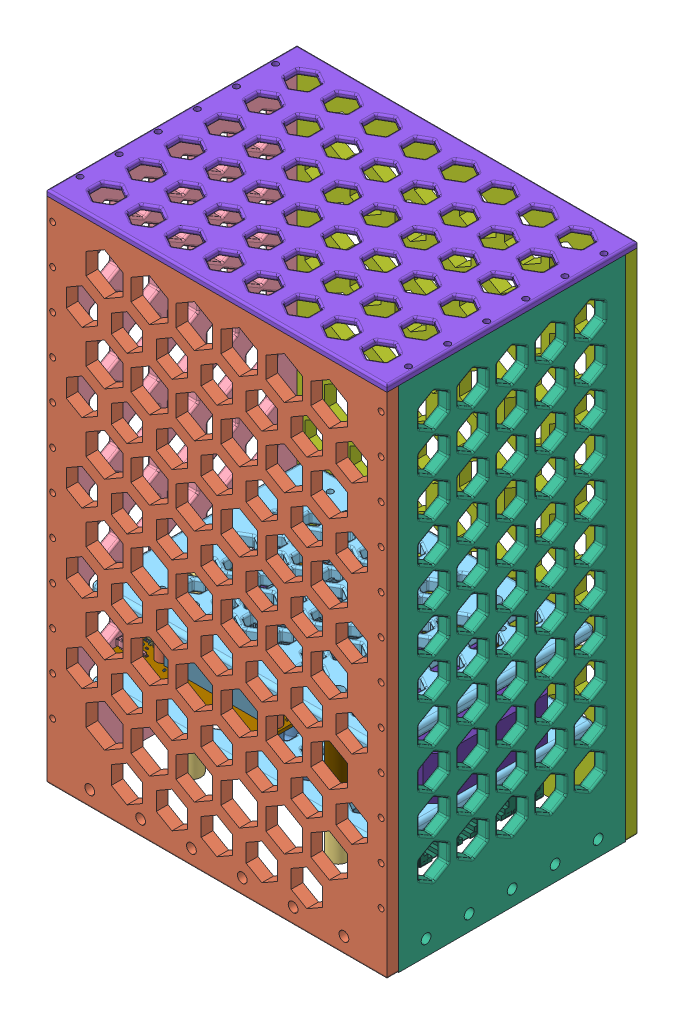
SolidWorks assembly upperbody, configuration 默认. Lengths in mm. (continued)
Components (placement in the parent): (continued)
- 交换机-1: 交换机 [默认] at (61.0275 78.8383 258.5616) x (0 0 1) z (0 -1 0) size (65.92 49.68 16.5)
  - LX-SWF502-2.step-1: LX-SWF502-2.step [Default] at (-129.5338 -11.9883 -6.5513) size (65.92 49.68 16.5)
    - RJEO-D19.step-1: RJEO-D19.step [Default] at (21.7657 41.0001 1.6) size (1.62 0.82 0.56)
      - LED0603N.step-1: LED0603N.step [Default] at origin size (1.62 0.82 0.56)
        - COMPOUND.step-1: COMPOUND.step [Default] at origin size (1.62 0.82 0.56)
    - RJEO-D2.step-1: RJEO-D2.step [Default] at (30.6411 41.0001 1.6) size (1.62 0.82 0.56)
      - LED0603N.step-1: LED0603N.step [Default] at origin size (1.62 0.82 0.56)
        - COMPOUND.step-1: COMPOUND.step [Default] at origin size (1.62 0.82 0.56)
    - RJEO-D20.step-1: RJEO-D20.step [Default] at (44.1334 41.0001 1.6) size (1.62 0.82 0.56)
      - LED0603N.step-1: LED0603N.step [Default] at origin size (1.62 0.82 0.56)
        - COMPOUND.step-1: COMPOUND.step [Default] at origin size (1.62 0.82 0.56)
    - RJEO-D21.step-1: RJEO-D21.step [Default] at (39.6501 41.0001 1.6) size (1.62 0.82 0.56)
      - LED0603N.step-1: LED0603N.step [Default] at origin size (1.62 0.82 0.56)
        - COMPOUND.step-1: COMPOUND.step [Default] at origin size (1.62 0.82 0.56)
    - RJEO-D22.step-1: RJEO-D22.step [Default] at (35.1271 41.0001 1.6) size (1.62 0.82 0.56)
      - LED0603N.step-1: LED0603N.step [Default] at origin size (1.62 0.82 0.56)
        - COMPOUND.step-1: COMPOUND.step [Default] at origin size (1.62 0.82 0.56)
    - RJEO-D1.step-1: RJEO-D1.step [Default] at (26.2147 41.0001 1.6) size (1.62 0.82 0.56)
      - LED0603N.step-1: LED0603N.step [Default] at origin size (1.62 0.82 0.56)
        - COMPOUND.step-1: COMPOUND.step [Default] at origin size (1.62 0.82 0.56)
    - RJEO-C10.step-1: RJEO-C10.step [Default] at (28.0001 37.4021 1.6) x (0 1 0) z (0 0 1) size (1 0.5 0.5)
      - 0402.step-1: 0402.step [Default] at origin size (1 0.5 0.5)
        - SOLID.step-1: SOLID.step [Default] at origin size (1 0.5 0.5)
    - RJEO-C11.step-1: RJEO-C11.step [Default] at (22.346 36.1431 1.6) x (-1 0 0) z (0 0 1) size (1 0.5 0.5)
      - 0402.step-1: 0402.step [Default] at origin size (1 0.5 0.5)
        - SOLID.step-1: SOLID.step [Default] at origin size (1 0.5 0.5)
    - RJEO-C13.step-1: RJEO-C13.step [Default] at (28.1391 26.6451 1.6) x (0 -1 0) z (0 0 1) size (1 0.5 0.5)
      - 0402.step-1: 0402.step [Default] at origin size (1 0.5 0.5)
        - SOLID.step-1: SOLID.step [Default] at origin size (1 0.5 0.5)
    - RJEO-C14.step-1: RJEO-C14.step [Default] at (32.6271 28.0611 1.6) x (0 -1 0) z (0 0 1) size (1 0.5 0.5)
      - 0402-1.step-1: 0402-1.step [Default] at origin size (1 0.5 0.5)
        - SOLID-0.step-1: SOLID-0.step [Default] at origin size (1 0.5 0.5)
    - RJEO-C15.step-1: RJEO-C15.step [Default] at (33.7611 35.9131 1.6) size (1 0.5 0.5)
      - 0402.step-1: 0402.step [Default] at origin size (1 0.5 0.5)
        - SOLID.step-1: SOLID.step [Default] at origin size (1 0.5 0.5)
    - RJEO-C16.step-1: RJEO-C16.step [Default] at (25.0001 37.5751 1.6) x (0 1 0) z (0 0 1) size (1 0.5 0.5)
      - 0402.step-1: 0402.step [Default] at origin size (1 0.5 0.5)
        - SOLID.step-1: SOLID.step [Default] at origin size (1 0.5 0.5)
    - RJEO-C17.step-1: RJEO-C17.step [Default] at (21.666 30.3191 1.6) x (-0.707107 -0.707107 0) z (0 0 1) size (1 0.5 0.5)
      - 0402.step-1: 0402.step [Default] at origin size (1 0.5 0.5)
        - SOLID.step-1: SOLID.step [Default] at origin size (1 0.5 0.5)
    - RJEO-C18.step-1: RJEO-C18.step [Default] at (23.917 26.8671 1.6) x (-0.707107 -0.707107 0) z (0 0 1) size (1 0.5 0.5)
      - 0402.step-1: 0402.step [Default] at origin size (1 0.5 0.5)
        - SOLID.step-1: SOLID.step [Default] at origin size (1 0.5 0.5)
    - RJEO-C19.step-1: RJEO-C19.step [Default] at (34.9891 39.2441 1.6) size (1 0.5 0.5)
      - 0402.step-1: 0402.step [Default] at origin size (1 0.5 0.5)
        - SOLID.step-1: SOLID.step [Default] at origin size (1 0.5 0.5)
    - RJEO-C2.step-1: RJEO-C2.step [Default] at (32.8971 20.6 1.6) x (0 1 0) z (0 0 1) size (1 0.5 0.5)
      - 0402.step-1: 0402.step [Default] at origin size (1 0.5 0.5)
        - SOLID.step-1: SOLID.step [Default] at origin size (1 0.5 0.5)
    - RJEO-C20.step-1: RJEO-C20.step [Default] at (31.5481 20.6 1.6) x (0 1 0) z (0 0 1) size (1 0.5 0.5)
      - 0402.step-1: 0402.step [Default] at origin size (1 0.5 0.5)
        - SOLID.step-1: SOLID.step [Default] at origin size (1 0.5 0.5)
    - RJEO-C25.step-1: RJEO-C25.step [Default] at (13.815 20.6 1.6) x (0 1 0) z (0 0 1) size (1 0.5 0.5)
      - 0402.step-1: 0402.step [Default] at origin size (1 0.5 0.5)
        - SOLID.step-1: SOLID.step [Default] at origin size (1 0.5 0.5)
    - RJEO-C37.step-1: RJEO-C37.step [Default] at (23.177 27.5921 1.6) x (-0.707107 -0.707107 0) z (0 0 1) size (1 0.5 0.5)
      - 0402.step-1: 0402.step [Default] at origin size (1 0.5 0.5)
        - SOLID.step-1: SOLID.step [Default] at origin size (1 0.5 0.5)
    - RJEO-C7.step-1: RJEO-C7.step [Default] at (34.7321 30.7291 1.6) x (0 -1 0) z (0 0 1) size (1 0.5 0.5)
      - 0402.step-1: 0402.step [Default] at origin size (1 0.5 0.5)
        - SOLID.step-1: SOLID.step [Default] at origin size (1 0.5 0.5)
    - RJEO-C8.step-1: RJEO-C8.step [Default] at (29.1961 26.6451 1.6) x (0 -1 0) z (0 0 1) size (1 0.5 0.5)
      - 0402.step-1: 0402.step [Default] at origin size (1 0.5 0.5)
        - SOLID.step-1: SOLID.step [Default] at origin size (1 0.5 0.5)
    - RJEO-C21.step-1: RJEO-C21.step [Default] at (5.908 27.1321 1.6) x (-1 0 0) z (0 0 1) size (1 0.5 0.5)
      - C0402.step-1: C0402.step [Default] at origin size (1 0.5 0.5)
        - SOLID-1.step-1: SOLID-1.step [Default] at origin size (1 0.5 0.5)
    - RJEO-C22.step-1: RJEO-C22.step [Default] at (6.552 21.19 1.6) size (1 0.5 0.5)
      - C0402.step-1: C0402.step [Default] at origin size (1 0.5 0.5)
        - SOLID-1.step-1: SOLID-1.step [Default] at origin size (1 0.5 0.5)
    - RJEO-C3.step-1: RJEO-C3.step [Default] at (32.5331 37.9101 1.6) x (0 1 0) z (0 0 1) size (1 0.5 0.5)
      - C0402.step-1: C0402.step [Default] at origin size (1 0.5 0.5)
        - SOLID-1.step-1: SOLID-1.step [Default] at origin size (1 0.5 0.5)
    - RJEO-C4.step-1: RJEO-C4.step [Default] at (18.817 32.7271 1.6) x (-1 0 0) z (0 0 1) size (1 0.5 0.5)
      - C0402.step-1: C0402.step [Default] at origin size (1 0.5 0.5)
        - SOLID-1.step-1: SOLID-1.step [Default] at origin size (1 0.5 0.5)
    - RJEO-C5.step-1: RJEO-C5.step [Default] at (18.81 37.8231 1.6) x (-1 0 0) z (0 0 1) size (1 0.5 0.5)
      - C0402.step-1: C0402.step [Default] at origin size (1 0.5 0.5)
        - SOLID-1.step-1: SOLID-1.step [Default] at origin size (1 0.5 0.5)
    - RJEO-C1.step-1: RJEO-C1.step [Default] at (51.3311 20.6 1.6) x (0 1 0) z (0 0 1) size (1 0.5 0.5)
      - 0402.step-1: 0402.step [Default] at origin size (1 0.5 0.5)
        - SOLID.step-1: SOLID.step [Default] at origin size (1 0.5 0.5)
    - RJEO-R11.step-1: RJEO-R11.step [Default] at (6.402 25.9921 1.6) x (-1 0 0) z (0 0 1) size (1 0.5 0.5)
      - 0402-2.step-1: 0402-2.step [Default] at origin size (1 0.5 0.5)
        - SOLID-2.step-1: SOLID-2.step [Default] at origin size (1 0.5 0.5)
    - RJEO-R12.step-1: RJEO-R12.step [Default] at (3.948 21.19 1.6) size (1 0.5 0.5)
      - 0402-2.step-1: 0402-2.step [Default] at origin size (1 0.5 0.5)
        - SOLID-2.step-1: SOLID-2.step [Default] at origin size (1 0.5 0.5)
    - RJEO-R13.step-1: RJEO-R13.step [Default] at (1.211 22.273 1.6) x (0 -1 0) z (0 0 1) size (1 0.5 0.5)
      - 0402-2.step-1: 0402-2.step [Default] at origin size (1 0.5 0.5)
        - SOLID-2.step-1: SOLID-2.step [Default] at origin size (1 0.5 0.5)
    - RJEO-R14.step-1: RJEO-R14.step [Default] at (2.295 24.326 1.6) x (0 -1 0) z (0 0 1) size (1 0.5 0.5)
      - 0402-2.step-1: 0402-2.step [Default] at origin size (1 0.5 0.5)
        - SOLID-2.step-1: SOLID-2.step [Default] at origin size (1 0.5 0.5)
    - RJEO-R15.step-1: RJEO-R15.step [Default] at (2.295 21.285 1.6) x (0 1 0) z (0 0 1) size (1 0.5 0.5)
      - 0402-2.step-1: 0402-2.step [Default] at origin size (1 0.5 0.5)
        - SOLID-2.step-1: SOLID-2.step [Default] at origin size (1 0.5 0.5)
    - RJEO-R2.step-1: RJEO-R2.step [Default] at (20.272 31.5191 1.6) size (1 0.5 0.5)
      - 0402-2.step-1: 0402-2.step [Default] at origin size (1 0.5 0.5)
        - SOLID-2.step-1: SOLID-2.step [Default] at origin size (1 0.5 0.5)
    - RJEO-R20.step-1: RJEO-R20.step [Default] at (26.4001 42.3001 1.6) size (1 0.5 0.5)
      - 0402-2.step-1: 0402-2.step [Default] at origin size (1 0.5 0.5)
        - SOLID-2.step-1: SOLID-2.step [Default] at origin size (1 0.5 0.5)
    - RJEO-R21.step-1: RJEO-R21.step [Default] at (31.0661 42.3001 1.6) size (1 0.5 0.5)
      - 0402-2.step-1: 0402-2.step [Default] at origin size (1 0.5 0.5)
        - SOLID-2.step-1: SOLID-2.step [Default] at origin size (1 0.5 0.5)
    - RJEO-R22.step-1: RJEO-R22.step [Default] at (35.6971 42.3001 1.6) size (1 0.5 0.5)
      - 0402-2.step-1: 0402-2.step [Default] at origin size (1 0.5 0.5)
        - SOLID-2.step-1: SOLID-2.step [Default] at origin size (1 0.5 0.5)
    - RJEO-R23.step-1: RJEO-R23.step [Default] at (40.2871 42.3001 1.6) size (1 0.5 0.5)
      - 0402-2.step-1: 0402-2.step [Default] at origin size (1 0.5 0.5)
        - SOLID-2.step-1: SOLID-2.step [Default] at origin size (1 0.5 0.5)
    - RJEO-R24.step-1: RJEO-R24.step [Default] at (45.0261 42.3001 1.6) size (1 0.5 0.5)
      - 0402-2.step-1: 0402-2.step [Default] at origin size (1 0.5 0.5)
        - SOLID-2.step-1: SOLID-2.step [Default] at origin size (1 0.5 0.5)
    - RJEO-R26.step-1: RJEO-R26.step [Default] at (21.524 42.3001 1.6) size (1 0.5 0.5)
      - 0402-2.step-1: 0402-2.step [Default] at origin size (1 0.5 0.5)
        - SOLID-2.step-1: SOLID-2.step [Default] at origin size (1 0.5 0.5)
    - RJEO-R3.step-1: RJEO-R3.step [Default] at (33.6221 38.4311 1.6) x (0 -1 0) z (0 0 1) size (1 0.5 0.5)
      - 0402-2.step-1: 0402-2.step [Default] at origin size (1 0.5 0.5)
        - SOLID-2.step-1: SOLID-2.step [Default] at origin size (1 0.5 0.5)
    - RJEO-R4.step-1: RJEO-R4.step [Default] at (30.3291 38.4071 1.6) x (0 -1 0) z (0 0 1) size (1 0.5 0.5)
      - 0402-2.step-1: 0402-2.step [Default] at origin size (1 0.5 0.5)
        - SOLID-2.step-1: SOLID-2.step [Default] at origin size (1 0.5 0.5)
    - RJEO-R5.step-1: RJEO-R5.step [Default] at (44.0581 42.3001 1.6) x (-1 0 0) z (0 0 1) size (1 0.5 0.5)
      - 0402-2.step-1: 0402-2.step [Default] at origin size (1 0.5 0.5)
        - SOLID-2.step-1: SOLID-2.step [Default] at origin size (1 0.5 0.5)
    - RJEO-R6.step-1: RJEO-R6.step [Default] at (39.2791 42.3001 1.6) x (-1 0 0) z (0 0 1) size (1 0.5 0.5)
      - 0402-2.step-1: 0402-2.step [Default] at origin size (1 0.5 0.5)
        - SOLID-2.step-1: SOLID-2.step [Default] at origin size (1 0.5 0.5)
    - RJEO-R7.step-1: RJEO-R7.step [Default] at (34.6091 42.3001 1.6) x (-1 0 0) z (0 0 1) size (1 0.5 0.5)
      - 0402-2.step-1: 0402-2.step [Default] at origin size (1 0.5 0.5)
        - SOLID-2.step-1: SOLID-2.step [Default] at origin size (1 0.5 0.5)
    - RJEO-R8.step-1: RJEO-R8.step [Default] at (30.0421 42.3001 1.6) x (-1 0 0) z (0 0 1) size (1 0.5 0.5)
      - 0402-2.step-1: 0402-2.step [Default] at origin size (1 0.5 0.5)
        - SOLID-2.step-1: SOLID-2.step [Default] at origin size (1 0.5 0.5)
    - RJEO-R9.step-1: RJEO-R9.step [Default] at (25.3031 42.3001 1.6) x (-1 0 0) z (0 0 1) size (1 0.5 0.5)
      - 0402-2.step-1: 0402-2.step [Default] at origin size (1 0.5 0.5)
        - SOLID-2.step-1: SOLID-2.step [Default] at origin size (1 0.5 0.5)
    - RJEO-R1.step-1: RJEO-R1.step [Default] at (31.4191 37.4141 1.6) x (0 1 0) z (0 0 1) size (1 0.5 0.5)
      - 0402-2.step-1: 0402-2.step [Default] at origin size (1 0.5 0.5)
        - SOLID-2.step-1: SOLID-2.step [Default] at origin size (1 0.5 0.5)
    - RJEO-JP1.step-1: RJEO-JP1.step [Default] at (12.001 40.0001 1.6) x (-1 0 0) z (0 0 1) size (7.5 5.9 10.6)
      - SIP2.step-1: SIP2.step [Default] at origin size (7.5 5.9 10.6)
        - COMPOUND-3.step-1: COMPOUND-3.step [Default] at origin size (7.5 5.9 10.6)
    - RJEO-DXFRM3.step-1: RJEO-DXFRM3.step [Default] at (21.989 19.3 1.6) x (-1 0 0) z (0 0 1) size (15.1 10 4.5)
      - NS892407B.step-1: NS892407B.step [Default] at origin size (15.1 10 4.5)
        - COMPOUND-4.step-1: COMPOUND-4.step [Default] at origin size (15.1 10 4.5)
    - RJEO-DXFRM1.step-1: RJEO-DXFRM1.step [Default] at (41.7141 19.3 1.6) x (-1 0 0) z (0 0 1) size (15.1 10 4.5)
      - NS892407B.step-1: NS892407B.step [Default] at origin size (15.1 10 4.5)
        - COMPOUND-4.step-1: COMPOUND-4.step [Default] at origin size (15.1 10 4.5)
    - RJEO-L2.step-1: RJEO-L2.step [Default] at (10.114 25.031 1.6) x (0 -1 0) z (0 0 1) size (4.4 4.2 2.1)
      - L10A.step-1: L10A.step [Default] at origin size (4.4 4.2 2.1)
        - SOLID-5.step-1: SOLID-5.step [Default] at origin size (4.4 4.2 2.1)
    - RJEO-TC4.step-1: RJEO-TC4.step [Default] at (4.629 32.6291 1.6) x (0 -1 0) z (0 0 1) size (6.6 7.8 7.75)
      - CAP-E-SMD-D6.3.step-1: CAP-E-SMD-D6.3.step [Default] at origin size (6.6 7.8 7.75)
        - SOLID-6.step-1: SOLID-6.step [Default] at origin size (6.6 7.8 7.75)
    - RJEO-TC1.step-1: RJEO-TC1.step [Default] at (16 28.8001 1.6) x (0 1 0) z (0 0 1) size (6.6 7.8 7.75)
      - CAP-E-SMD-D6.3.step-1: CAP-E-SMD-D6.3.step [Default] at origin size (6.6 7.8 7.75)
        - SOLID-6.step-1: SOLID-6.step [Default] at origin size (6.6 7.8 7.75)
    - RJEO-TRS1.step-1: RJEO-TRS1.step [Default] at (41.5201 33.5001 1.6) x (0 -1 0) z (0 0 1) size (12.7 9.5 5.95)
      - RJ45-8PIN.step-1: RJ45-8PIN.step [Default] at origin size (12.7 9.5 5.95)
        - COMPOUND-7.step-1: COMPOUND-7.step [Default] at origin size (12.7 9.5 5.95)
    - RJEO-Y6.step-1: RJEO-Y6.step [Default] at (18.772 35.3521 1.6) x (0 1 0) z (0 0 1) size (3.2 2.5 0.72)
      - SM091.step-1: SM091.step [Default] at origin size (3.2 2.5 0.72)
        - SOLID-8.step-1: SOLID-8.step [Default] at origin size (3.2 2.5 0.72)
    - RJEO-U1.step-1: RJEO-U1.step [Default] at (6.457 22.482 1.6) x (0 1 0) z (0 0 1) size (2.88 2.79 1.64)
      - SOT23-6.step-1: SOT23-6.step [Default] at origin size (2.88 2.79 1.64)
        - COMPOUND-9.step-1: COMPOUND-9.step [Default] at origin size (2.88 2.79 1.64)
    - RJEO-U2.step-1: RJEO-U2.step [Default] at (28.0001 32.0001 1.6) x (-1 0 0) z (0 0 1) size (6 6 0.85)
      - QFN48_04_EPAD.step-1: QFN48_04_EPAD.step [Default] at origin size (6 6 0.85)
        - COMPOUND-10.step-1: COMPOUND-10.step [Default] at origin size (6 6 0.85)
    - RJEO-H6.step-1: RJEO-H6.step [Default] at (56.8961 40.8691 1.6) x (-1 0 0) z (0 0 1) size (16.45 16.05 15.8)
      - RJ45-1X1-B.step-1: RJ45-1X1-B.step [Default] at origin size (16.45 16.05 15.8)
        - COMPOUND-11.step-1: COMPOUND-11.step [Default] at origin size (16.45 16.05 15.8)
    - RJEO-H7.step-1: RJEO-H7.step [Default] at (33.1521 2.093 1.6) size (63.76 15.76 16.2)
      - RJ45-1X4-B.step-1: RJ45-1X4-B.step [Default] at origin size (63.76 15.76 16.2)
        - COMPOUND-12.step-1: COMPOUND-12.step [Default] at origin size (63.76 15.76 16.2)
    - Board.step-1: Board.step [Default] at origin size (65.92 43.41 1.6)
- 转压-1: 转压 [默认] at (54.0084 99.9888 161.9625) x (-1 0 0) z (0 0 -1) size (57.6 22 63.7)
- ctrlbox-3: ctrlbox [默认] at (5.0084 130.5588 162) size (148 6 110)
- M6螺柱35-3: M6螺柱35 [默认] at (42.5084 93.9888 122) x (0.932693 0 -0.360672) z (0.360672 0 0.932693) size (10 35 10)
- M6螺柱35-4: M6螺柱35 [默认] at (42.5084 93.9888 202) x (0.513313 0 -0.858202) z (0.858202 0 0.513313) size (10 35 10)
- M3螺柱10-5: M3螺柱10 [默认] at (10.5084 93.9888 116) size (6 10 6)
- M3螺柱10-6: M3螺柱10 [默认] at (-47.4916 93.9888 116) size (6 10 6)
- M3螺柱10-7: M3螺柱10 [默认] at (-47.4916 93.9888 202) size (6 10 6)
- M3螺柱10-8: M3螺柱10 [默认] at (10.5084 93.9888 202) size (6 10 6)
- M3螺柱25-1: M3螺柱25 [默认] at (10.5084 105.5588 116) x (0.994103 0 0.108442) z (-0.108442 0 0.994103) size (6 25 6)
- M3螺柱25-2: M3螺柱25 [默认] at (-47.4916 105.5588 116) x (0.999732 0 0.023161) z (-0.023161 0 0.999732) size (6 25 6)
- M3螺柱25-3: M3螺柱25 [默认] at (-47.4916 105.5588 202) x (0.999732 0 0.023161) z (-0.023161 0 0.999732) size (6 25 6)
- M3螺柱25-4: M3螺柱25 [默认] at (10.5084 105.5588 202) x (0.999732 0 0.023161) z (-0.023161 0 0.999732) size (6 25 6)
- M4螺柱6-1: M4螺柱6 [默认] at (51.5084 93.9888 188.9625) x (0.999997 0 -0.002414) z (0.002414 0 0.999997) size (6 6 6)
- M4螺柱6-2: M4螺柱6 [默认] at (51.5084 93.9888 134.9625) x (0.9996 0 -0.02829) z (0.02829 0 0.9996) size (6 6 6)
Mates (geometry in assembly coordinates):
- Coincident1: coincident anti-aligned: plane of crotch-1 through (85.5084 62.9888 162) normal (0 1 0); plane of imu-1 through (4.5084 62.9888 136) normal (0 -1 0)
- Concentric1: concentric anti-aligned: cylinder of crotch-1 through (4.5084 42.9888 116.5) axis (0 1 0) radius 1.5; cylinder of imu-1 through (4.5084 66.9888 116.5) axis (0 -1 0) radius 1.6
- Concentric2: concentric anti-aligned: cylinder of crotch-1 through (-12.4916 42.9888 155.5) axis (0 1 0) radius 1.5; cylinder of imu-1 through (-12.4916 66.9888 155.5) axis (0 -1 0) radius 1.6
- Coincident4: coincident anti-aligned: plane of crotch-1 through (85.5084 -17.0112 220) normal (0 0 1); plane of front-1 through (4.5084 194.9888 220) normal (0 0 -1)
- Concentric3: concentric aligned: cylinder of crotch-1 through (-60.4916 52.9888 213) axis (0 0 1) radius 2.5; cylinder of front-1 through (-60.4916 52.9888 220) axis (0 0 1) radius 2.5
- Concentric4: concentric aligned: cylinder of crotch-1 through (69.5084 52.9888 213) axis (0 0 1) radius 2.5; cylinder of front-1 through (69.5084 52.9888 220) axis (0 0 1) radius 2.5
- Concentric5: concentric anti-aligned: cylinder of crotch-1 through (42.5084 42.9888 122) axis (0 1 0) radius 3; cylinder of M8螺柱-1 through (42.5084 87.9888 122) axis (0 -1 0) radius 3
- Coincident6: coincident anti-aligned: plane of crotch-1 through (85.5084 62.9888 162) normal (0 1 0); plane of M8螺柱-1 through (42.5084 62.9888 122) normal (0 -1 0)
- Concentric6: concentric anti-aligned: cylinder of crotch-1 through (42.5084 42.9888 202) axis (0 1 0) radius 3; cylinder of M8螺柱-2 through (42.5084 87.9888 202) axis (0 -1 0) radius 3
- Coincident7: coincident anti-aligned: plane of crotch-1 through (85.5084 62.9888 162) normal (0 1 0); plane of M8螺柱-2 through (42.5084 62.9888 202) normal (0 -1 0)
- Concentric7: concentric anti-aligned: cylinder of crotch-1 through (-32.4916 42.9888 122) axis (0 1 0) radius 3; cylinder of M8螺柱-3 through (-32.4916 87.9888 122) axis (0 -1 0) radius 3
- Coincident8: coincident anti-aligned: plane of crotch-1 through (85.5084 62.9888 162) normal (0 1 0); plane of M8螺柱-3 through (-32.4916 62.9888 122) normal (0 -1 0)
- Concentric8: concentric anti-aligned: cylinder of crotch-1 through (-32.4916 42.9888 202) axis (0 1 0) radius 3; cylinder of M8螺柱-4 through (-32.4916 87.9888 202) axis (0 -1 0) radius 5
- Coincident9: coincident anti-aligned: plane of crotch-1 through (85.5084 62.9888 162) normal (0 1 0); plane of M8螺柱-4 through (-32.4916 62.9888 202) normal (0 -1 0)
- Concentric9: concentric anti-aligned: cylinder of crotch-1 through (-69.4916 52.9888 184) axis (-1 0 0) radius 2.5; cylinder of left-1 through (-82.4916 52.9888 184) axis (1 0 0) radius 2.5
- Concentric10: concentric anti-aligned: cylinder of crotch-1 through (-69.4916 52.9888 140) axis (-1 0 0) radius 2.5; cylinder of left-1 through (-82.4916 52.9888 140) axis (1 0 0) radius 2.5
- Coincident10: coincident anti-aligned: plane of crotch-1 through (-76.4916 -17.0112 162) normal (-1 0 0); plane of left-1 through (-76.4916 204.9888 162) normal (1 0 0)
- Concentric11: concentric anti-aligned: cylinder of crotch-1 through (78.5084 52.9888 118) axis (1 0 0) radius 2.5; cylinder of right-1 through (91.5084 52.9888 118) axis (-1 0 0) radius 2.5
- Concentric12: concentric anti-aligned: cylinder of crotch-1 through (78.5084 52.9888 206) axis (1 0 0) radius 2.5; cylinder of right-1 through (91.5084 52.9888 206) axis (-1 0 0) radius 2.5
- Coincident11: coincident anti-aligned: plane of crotch-1 through (85.5084 -17.0112 162) normal (1 0 0); plane of right-1 through (85.5084 204.9888 162) normal (-1 0 0)
- Concentric13: concentric anti-aligned: cylinder of M8螺柱-1 through (42.5084 87.9888 122) axis (0 -1 0) radius 3; cylinder of ctrlbox-2 through (42.5084 87.9888 122) axis (0 1 0) radius 3
- Concentric14: concentric anti-aligned: cylinder of M8螺柱-4 through (-32.4916 87.9888 202) axis (0 -1 0) radius 3; cylinder of ctrlbox-2 through (-32.4916 87.9888 202) axis (0 1 0) radius 3
- Coincident13: coincident anti-aligned: plane of M8螺柱-3 through (-32.4916 87.9888 122) normal (0 1 0); plane of ctrlbox-2 through (5.0084 87.9888 162) normal (0 -1 0)
- Concentric22: concentric anti-aligned: cylinder of crotch-1 through (69.5084 52.9888 111) axis (0 0 -1) radius 2.5; cylinder of back-2 through (69.5084 52.9888 98) axis (0 0 1) radius 2.5
- Concentric23: concentric anti-aligned: cylinder of crotch-1 through (-60.4916 52.9888 111) axis (0 0 -1) radius 2.5; cylinder of back-2 through (-60.4916 52.9888 98) axis (0 0 1) radius 2.5
- Coincident22: coincident anti-aligned: plane of crotch-1 through (85.5084 -17.0112 104) normal (0 0 -1); plane of back-2 through (4.5084 194.9888 104) normal (0 0 1)
- Concentric39: concentric aligned: cylinder of right-1 through (88.5084 296.9888 212) axis (0 1 0) radius 1.5; cylinder of top-1 through (88.5084 304.9888 212) axis (0 1 0) radius 1.25
- Concentric40: concentric aligned: cylinder of left-1 through (-79.4916 296.9888 212) axis (0 1 0) radius 1.5; cylinder of top-1 through (-79.4916 304.9888 212) axis (0 1 0) radius 1.25
- Coincident26: coincident anti-aligned: plane of front-1 through (4.5084 304.9888 220) normal (0 1 0); plane of top-1 through (4.5084 304.9888 162) normal (0 -1 0)
- Parallel11: parallel anti-aligned: plane of battery-1 through (73.2915 136.5588 99.1011) normal (0 -1 0); plane of ctrlbox-2 through (5.0084 93.9888 162) normal (0 1 0)
- Parallel12: parallel aligned: plane of crotch-1 through (85.5084 -17.0112 104) normal (0 0 -1); plane of battery-1 through (3.2915 206.5588 99.1011) normal (0 0 -1)
- Concentric44: concentric aligned: cylinder of ctrlbox-2 through (10.5084 83.9888 202) axis (0 1 0) radius 1.5; cylinder of jetsonnano-1/675_13541_batuu_dev_kit_top_ass_asm.stp-1/642-13541_BATUU_SYS_BOM_ASM.stp-1/600-13542-BASE-A02_ASM.stp-1/600-13542-BASE-A02.stp-1 through (10.5084 103.9888 202) axis (0 1 0) radius 1.375
- Concentric45: concentric aligned: cylinder of ctrlbox-2 through (10.5084 83.9888 116) axis (0 1 0) radius 1.5; cylinder of jetsonnano-1/675_13541_batuu_dev_kit_top_ass_asm.stp-1/642-13541_BATUU_SYS_BOM_ASM.stp-1/600-13542-BASE-A02_ASM.stp-1/600-13542-BASE-A02.stp-1 through (10.5084 103.9888 116) axis (0 1 0) radius 1.375
- Concentric62: concentric aligned: cylinder of ctrlbox-2 through (46.7384 83.9888 192.09) axis (0 1 0) radius 1.5; cylinder of 交换机-1/LX-SWF502-2.step-1/Board.step-1 through (46.7384 85.3897 192.09) axis (0 1 0) radius 1.5
- Parallel17: parallel aligned: plane of ctrlbox-2 through (-68.9916 93.9888 217) normal (0 0 1); plane of 交换机-1/LX-SWF502-2.step-1/Board.step-1 through (29.7887 85.3897 194.9996) normal (0 0 1)
- Parallel18: parallel aligned: plane of ctrlbox-2 through (79.0084 93.9888 217) normal (1 0 0); plane of 交换机-1/LX-SWF502-2.step-1/Board.step-1 through (73.202 85.3897 194.9996) normal (1 0 0)
- Parallel19: parallel anti-aligned: plane of ctrlbox-2 through (5.0084 93.9888 162) normal (0 1 0); plane of 转压-1 through (54.0084 99.9888 161.9625) normal (0 -1 0)
- Parallel20: parallel aligned: plane of ctrlbox-2 through (79.0084 93.9888 217) normal (1 0 0); plane of 转压-1 through (82.8084 121.9888 188.8125) normal (1 0 0)
- Coincident45: coincident anti-aligned: plane of battery-1 through (73.2915 136.5588 99.1011) normal (0 -1 0); plane of ctrlbox-3 through (5.0084 136.5588 162) normal (0 1 0)
- Concentric69: concentric anti-aligned: cylinder of ctrlbox-2 through (42.5084 87.9888 122) axis (0 1 0) radius 3; cylinder of M6螺柱35-3 through (42.5084 128.9888 122) axis (0 -1 0) radius 3
- Coincident46: coincident anti-aligned: plane of ctrlbox-2 through (5.0084 93.9888 162) normal (0 1 0); plane of M6螺柱35-3 through (42.5084 93.9888 122) normal (0 -1 0)
- Concentric70: concentric anti-aligned: cylinder of ctrlbox-2 through (42.5084 87.9888 202) axis (0 1 0) radius 3; cylinder of M6螺柱35-4 through (42.5084 128.9888 202) axis (0 -1 0) radius 3
- Coincident47: coincident anti-aligned: plane of ctrlbox-2 through (5.0084 93.9888 162) normal (0 1 0); plane of M6螺柱35-4 through (42.5084 93.9888 202) normal (0 -1 0)
- Concentric71: concentric anti-aligned: cylinder of jetsonnano-1/675_13541_batuu_dev_kit_top_ass_asm.stp-1/642-13541_BATUU_SYS_BOM_ASM.stp-1/600-13542-BASE-A02_ASM.stp-1/600-13542-BASE-A02.stp-1 through (10.5084 103.9888 116) axis (0 1 0) radius 1.375; cylinder of M3螺柱10-5 through (10.5084 103.9888 116) axis (0 -1 0) radius 1.5
- Coincident48: coincident anti-aligned: plane of ctrlbox-2 through (5.0084 93.9888 162) normal (0 1 0); plane of M3螺柱10-5 through (10.5084 93.9888 116) normal (0 -1 0)
- Coincident49: coincident anti-aligned: plane of jetsonnano-1/675_13541_batuu_dev_kit_top_ass_asm.stp-1/642-13541_BATUU_SYS_BOM_ASM.stp-1/600-13542-BASE-A02_ASM.stp-1/600-13542-BASE-A02.stp-1 through (-47.4916 103.9888 116) normal (0 -1 0); plane of M3螺柱10-5 through (10.5084 103.9888 116) normal (0 1 0)
- Concentric72: concentric anti-aligned: cylinder of ctrlbox-2 through (-47.4916 83.9888 116) axis (0 1 0) radius 1.5; cylinder of M3螺柱10-6 through (-47.4916 103.9888 116) axis (0 -1 0) radius 1.5
- Coincident50: coincident anti-aligned: plane of jetsonnano-1/675_13541_batuu_dev_kit_top_ass_asm.stp-1/642-13541_BATUU_SYS_BOM_ASM.stp-1/600-13542-BASE-A02_ASM.stp-1/600-13542-BASE-A02.stp-1 through (-47.4916 103.9888 116) normal (0 -1 0); plane of M3螺柱10-6 through (-47.4916 103.9888 116) normal (0 1 0)
- Concentric73: concentric anti-aligned: cylinder of jetsonnano-1/675_13541_batuu_dev_kit_top_ass_asm.stp-1/642-13541_BATUU_SYS_BOM_ASM.stp-1/600-13542-BASE-A02_ASM.stp-1/600-13542-BASE-A02.stp-1 through (-47.4916 103.9888 202) axis (0 1 0) radius 1.375; cylinder of M3螺柱10-7 through (-47.4916 103.9888 202) axis (0 -1 0) radius 1.5
- Coincident51: coincident anti-aligned: plane of ctrlbox-2 through (5.0084 93.9888 162) normal (0 1 0); plane of M3螺柱10-7 through (-47.4916 93.9888 202) normal (0 -1 0)
- Concentric74: concentric anti-aligned: cylinder of jetsonnano-1/675_13541_batuu_dev_kit_top_ass_asm.stp-1/642-13541_BATUU_SYS_BOM_ASM.stp-1/600-13542-BASE-A02_ASM.stp-1/600-13542-BASE-A02.stp-1 through (10.5084 103.9888 202) axis (0 1 0) radius 1.375; cylinder of M3螺柱10-8 through (10.5084 103.9888 202) axis (0 -1 0) radius 1.5
- Coincident52: coincident anti-aligned: plane of jetsonnano-1/675_13541_batuu_dev_kit_top_ass_asm.stp-1/642-13541_BATUU_SYS_BOM_ASM.stp-1/600-13542-BASE-A02_ASM.stp-1/600-13542-BASE-A02.stp-1 through (-47.4916 103.9888 116) normal (0 -1 0); plane of M3螺柱10-8 through (10.5084 103.9888 202) normal (0 1 0)
- Concentric75: concentric anti-aligned: cylinder of jetsonnano-1/675_13541_batuu_dev_kit_top_ass_asm.stp-1/642-13541_BATUU_SYS_BOM_ASM.stp-1/600-13542-BASE-A02_ASM.stp-1/600-13542-BASE-A02.stp-1 through (10.5084 103.9888 116) axis (0 1 0) radius 1.375; cylinder of M3螺柱25-1 through (10.5084 130.5588 116) axis (0 -1 0) radius 1.5
- Coincident53: coincident anti-aligned: plane of jetsonnano-1/675_13541_batuu_dev_kit_top_ass_asm.stp-1/642-13541_BATUU_SYS_BOM_ASM.stp-1/600-13542-BASE-A02_ASM.stp-1/600-13542-BASE-A02.stp-1 through (-47.4916 105.5588 116) normal (0 1 0); plane of M3螺柱25-1 through (10.5084 105.5588 116) normal (0 -1 0)
- Concentric76: concentric anti-aligned: cylinder of jetsonnano-1/675_13541_batuu_dev_kit_top_ass_asm.stp-1/642-13541_BATUU_SYS_BOM_ASM.stp-1/600-13542-BASE-A02_ASM.stp-1/600-13542-BASE-A02.stp-1 through (-47.4916 103.9888 116) axis (0 1 0) radius 1.375; cylinder of M3螺柱25-2 through (-47.4916 130.5588 116) axis (0 -1 0) radius 1.5
- Coincident54: coincident anti-aligned: plane of jetsonnano-1/675_13541_batuu_dev_kit_top_ass_asm.stp-1/642-13541_BATUU_SYS_BOM_ASM.stp-1/600-13542-BASE-A02_ASM.stp-1/600-13542-BASE-A02.stp-1 through (-47.4916 105.5588 116) normal (0 1 0); plane of M3螺柱25-2 through (-47.4916 105.5588 116) normal (0 -1 0)
- Concentric77: concentric anti-aligned: cylinder of jetsonnano-1/675_13541_batuu_dev_kit_top_ass_asm.stp-1/642-13541_BATUU_SYS_BOM_ASM.stp-1/600-13542-BASE-A02_ASM.stp-1/600-13542-BASE-A02.stp-1 through (-47.4916 103.9888 202) axis (0 1 0) radius 1.375; cylinder of M3螺柱25-3 through (-47.4916 130.5588 202) axis (0 -1 0) radius 1.5
- Coincident55: coincident anti-aligned: plane of ctrlbox-3 through (5.0084 130.5588 162) normal (0 -1 0); plane of M3螺柱25-3 through (-47.4916 130.5588 202) normal (0 1 0)
- Coincident56: coincident anti-aligned: plane of jetsonnano-1/675_13541_batuu_dev_kit_top_ass_asm.stp-1/642-13541_BATUU_SYS_BOM_ASM.stp-1/600-13542-BASE-A02_ASM.stp-1/600-13542-BASE-A02.stp-1 through (-47.4916 105.5588 116) normal (0 1 0); plane of M3螺柱25-3 through (-47.4916 105.5588 202) normal (0 -1 0)
- Concentric78: concentric anti-aligned: cylinder of jetsonnano-1/675_13541_batuu_dev_kit_top_ass_asm.stp-1/642-13541_BATUU_SYS_BOM_ASM.stp-1/600-13542-BASE-A02_ASM.stp-1/600-13542-BASE-A02.stp-1 through (10.5084 103.9888 202) axis (0 1 0) radius 1.375; cylinder of M3螺柱25-4 through (10.5084 130.5588 202) axis (0 -1 0) radius 1.5
- Coincident57: coincident anti-aligned: plane of ctrlbox-3 through (5.0084 130.5588 162) normal (0 -1 0); plane of M3螺柱25-4 through (10.5084 130.5588 202) normal (0 1 0)
- Concentric79: concentric anti-aligned: cylinder of ctrlbox-3 through (-47.4916 126.5588 116) axis (0 1 0) radius 1.5; cylinder of M3螺柱25-2 through (-47.4916 130.5588 116) axis (0 -1 0) radius 1.5
- Concentric80: concentric anti-aligned: cylinder of ctrlbox-3 through (-47.4916 126.5588 202) axis (0 1 0) radius 1.5; cylinder of M3螺柱25-3 through (-47.4916 130.5588 202) axis (0 -1 0) radius 1.5
- Coincident58: coincident anti-aligned: plane of battery-1 through (73.2915 136.5588 99.1011) normal (0 -1 0); plane of ctrlbox-3 through (5.0084 136.5588 162) normal (0 1 0)
- Concentric81: concentric anti-aligned: cylinder of ctrlbox-2 through (51.5084 83.9888 188.9625) axis (0 1 0) radius 2; cylinder of 转压-1 through (51.5084 121.9888 188.9625) axis (0 -1 0) radius 3.25
- Concentric82: concentric anti-aligned: cylinder of ctrlbox-2 through (51.5084 83.9888 134.9625) axis (0 1 0) radius 2; cylinder of 转压-1 through (51.5084 121.9888 134.9625) axis (0 -1 0) radius 3.25
- Concentric83: concentric anti-aligned: cylinder of ctrlbox-2 through (51.5084 83.9888 188.9625) axis (0 1 0) radius 2; cylinder of M4螺柱6 - 副本-1 through (51.5084 99.9888 188.9625) axis (0 -1 0) radius 2
- Coincident59: coincident anti-aligned: plane of ctrlbox-2 through (5.0084 93.9888 162) normal (0 1 0); plane of M4螺柱6 - 副本-1 through (51.5084 93.9888 188.9625) normal (0 -1 0)
- Coincident60: coincident anti-aligned: plane of 转压-1 through (54.0084 99.9888 161.9625) normal (0 -1 0); plane of M4螺柱6 - 副本-1 through (51.5084 99.9888 188.9625) normal (0 1 0)
- Concentric84: concentric aligned: cylinder of 转压-1 through (51.5084 121.9888 134.9625) axis (0 -1 0) radius 3.25; cylinder of M4螺柱6 - 副本-2 through (51.5084 99.9888 134.9625) axis (0 -1 0) radius 2
- Coincident61: coincident anti-aligned: plane of ctrlbox-2 through (5.0084 93.9888 162) normal (0 1 0); plane of M4螺柱6 - 副本-2 through (51.5084 93.9888 134.9625) normal (0 -1 0)
